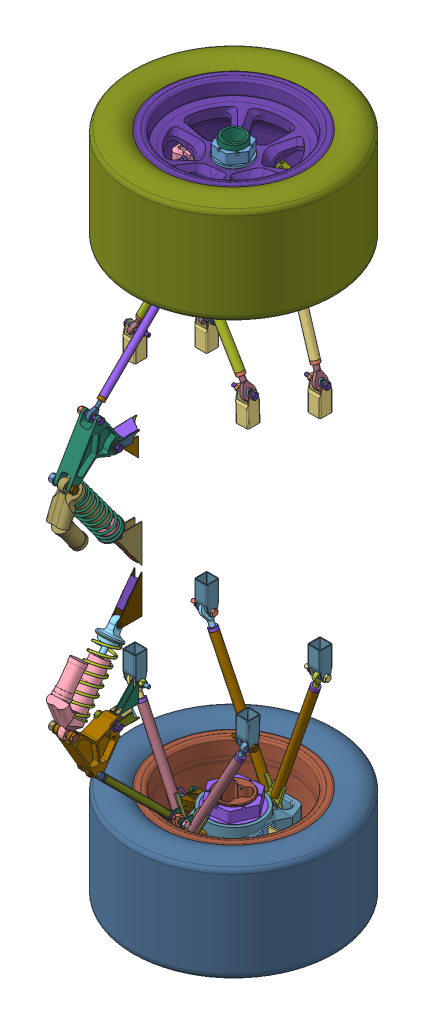
SolidWorks assembly UN-A1001-AB-Rear Unsprung Assembly, configuration Default. Lengths in mm.
Overall size (411.48 1363.58 600.2).
282 component instances, 147 part files, 8 mates.
Components (placement in the parent):
- SP-A0200-AH-Rear Axle Assembly-1: SP-A0200-AH-Rear Axle Assembly [Default] at origin size (274.88 563.57 484.64)
  - SP-AA-Rear Lower A-Arm^SP-A0200-AH-Rear Axle Assembly-1: SP-AA-Rear Lower A-Arm^SP-A0200-AH-Rear Axle Assembly [Default] at (0 -0.399 0.6588) x (1 0 0) z (0 0.002866 0.999996) size (222.76 290.57 36.42) (virtual)
    - SP-Lower Apex Rear-1: SP-Lower Apex Rear [Default] at (-792.4265 549.6462 121.5417) x (-0.932505 -0.360479 0.022123) z (0 -0.061256 -0.998122) size (54.94 63.8 9.53)
    - MirrorFS-MALE ROD END UNF-3A, 0.3125x24-0.25D (XAM-4)1-1: MirrorFS-MALE ROD END UNF-3A, 0.3125x24-0.25D (XAM-4)1 [Default] at (-906.7265 255.0788 139.6197) x (0.932505 -0.360479 0.022123) z (-0.361157 -0.930754 0.057121)
    - MirrorFS-MALE ROD END UNF-3A, 0.3125x24-0.25D (XAM-4)1-2: MirrorFS-MALE ROD END UNF-3A, 0.3125x24-0.25D (XAM-4)1 [Default] at (-678.1265 255.0788 139.6197) x (0.932505 0.360479 -0.022123) z (0.361157 -0.930754 0.057121)
    - SP-10003-AB-Threaded Insert-1: SP-10003-AB-Threaded Insert [A-Arm] at (-890.6731 296.4508 137.0806) x (0.932505 -0.360479 0.022123) z (-0.361157 -0.930754 0.057121) size (15.88 15.88 15.88)
    - SP-10003-AB-Threaded Insert-2: SP-10003-AB-Threaded Insert [A-Arm] at (-694.18 296.4508 137.0806) x (0.932505 0.360479 -0.022123) z (0.361157 -0.930754 0.057121) size (15.88 15.88 15.88)
    - SP-Rear Lower A-Arm Tube-1: SP-Rear Lower A-Arm Tube [Default] at (-838.6322 430.5677 128.8497) x (-0.361157 -0.930754 0.057121) z (0 -0.061256 -0.998122) size (257.84 15.88 15.88)
    - SP-Rear Lower A-Arm Tube-2: SP-Rear Lower A-Arm Tube [Default] at (-746.2209 430.5677 128.8497) x (0.361157 -0.930754 0.057121) z (0 0.061256 0.998122) size (257.84 15.88 15.88)
    - FS-HIGH MISALIGN SPHERICAL BEARING, 0.375-0.906D (3072-6G)-1: FS-HIGH MISALIGN SPHERICAL BEARING, 0.375-0.906D (3072-6G) [Default] at (-792.4265 549.6462 121.5417) x (-0.932505 0.360479 -0.022123) z (-0.361157 -0.930754 0.057121) size (26.46 21.71 26.13)
      - Race^FS-HIGH MISALIGN SPHERICAL BEARING, 0.375-0.906D (3072-6G)-1: Race^FS-HIGH MISALIGN SPHERICAL BEARING, 0.375-0.906D (3072-6G) [Default] at origin size (23.01 8.76 23.01) (virtual)
      - Ball^FS-HIGH MISALIGN SPHERICAL BEARING, 0.375-0.906D (3072-6G)-1: Ball^FS-HIGH MISALIGN SPHERICAL BEARING, 0.375-0.906D (3072-6G) [Default] x (0.359576 -0.008176 0.93308) z (-0.932238 -0.046516 0.358844) size (19.84 20.65 19.84) (virtual)
  - SP-AA-Rear Upper A-Arm^SP-A0200-AH-Rear Axle Assembly-1: SP-AA-Rear Upper A-Arm^SP-A0200-AH-Rear Axle Assembly [Default] at (-38.1 -1.9308 1.9372) x (1 0 0) z (0 0.00685 0.999977) size (216 215.55 29.43) (virtual)
    - SP-Upper Apex Rear-1: SP-Upper Apex Rear [Default] at (-755.8405 523.8827 293.8505) x (0.884705 -0.465567 -0.023329) z (0 -0.050046 0.998747) size (76.45 83.12 9.53)
    - MirrorFS-MALE ROD END UNF-3A, 0.3125x24-0.25D (XAM-4)1-1: MirrorFS-MALE ROD END UNF-3A, 0.3125x24-0.25D (XAM-4)1 [Default] at (-870.1405 307.2255 282.9942) x (0.884705 -0.465567 -0.023329) z (-0.466151 -0.883596 -0.044276)
    - MirrorFS-MALE ROD END UNF-3A, 0.3125x24-0.25D (XAM-4)1-2: MirrorFS-MALE ROD END UNF-3A, 0.3125x24-0.25D (XAM-4)1 [Default] at (-641.5405 307.2255 282.9942) x (0.884705 0.465567 0.023329) z (0.466151 -0.883596 -0.044276)
    - SP-10003-AB-Threaded Insert-1: SP-10003-AB-Threaded Insert [A-Arm] at (-849.4201 346.5014 284.9623) x (0.884705 -0.465567 -0.023329) z (-0.466151 -0.883596 -0.044276) size (15.88 15.88 15.88)
    - SP-10003-AB-Threaded Insert-2: SP-10003-AB-Threaded Insert [A-Arm] at (-662.261 346.5014 284.9623) x (0.884705 0.465567 0.023329) z (0.466151 -0.883596 -0.044276) size (15.88 15.88 15.88)
    - SP-Rear Upper A-Arm Tube-1: SP-Rear Upper A-Arm Tube [Default] at (-812.9905 415.5541 288.4224) x (0.466151 0.883596 0.044276) z (0.884705 -0.465567 -0.023329) size (186.28 15.88 15.88)
    - SP-Rear Upper A-Arm Tube-2: SP-Rear Upper A-Arm Tube [Default] at (-698.6905 415.5541 288.4224) x (-0.466151 0.883596 0.044276) z (0.884705 0.465567 0.023329) size (186.28 15.88 15.88)
    - FS-HIGH MISALIGN SPHERICAL BEARING, 0.375-0.906D (3072-6G)-1: FS-HIGH MISALIGN SPHERICAL BEARING, 0.375-0.906D (3072-6G) [Default] at (-755.8405 523.8827 293.8505) x (0.884705 -0.465567 -0.023329) z (-0.466151 -0.883596 -0.044276) size (26.46 21.71 26.13)
      - Race^FS-HIGH MISALIGN SPHERICAL BEARING, 0.375-0.906D (3072-6G)-1: Race^FS-HIGH MISALIGN SPHERICAL BEARING, 0.375-0.906D (3072-6G) [Default] at origin size (23.01 8.76 23.01) (virtual)
      - Ball^FS-HIGH MISALIGN SPHERICAL BEARING, 0.375-0.906D (3072-6G)-1: Ball^FS-HIGH MISALIGN SPHERICAL BEARING, 0.375-0.906D (3072-6G) [Default] x (0.359576 -0.008176 0.93308) z (-0.932238 -0.046516 0.358844) size (19.84 20.65 19.84) (virtual)
  - Assem8^SP-A0200-AH-Rear Axle Assembly-1: Assem8^SP-A0200-AH-Rear Axle Assembly [Default] at (-1592.9214 814.7933 712.2762) x (-0.999891 -0.01037 0.010464) z (0.012143 -0.982316 0.186836) size (17.98 166.51 230.13) (virtual)
    - Part2^Assem8_SP-A0200-AH-Rear Axle Assembly-1: Part2^Assem8_SP-A0200-AH-Rear Axle Assembly [Default] at origin size (15.39 113.92 157.78) (virtual)
    - SP-10003-AC-Threaded Insert-2: SP-10003-AC-Threaded Insert [AM-4 Rod End Thread] at (-799.064 427.6015 294.0449) x (-0.999891 -0.008342 0.012143) z (-0.014733 0.566176 -0.824153) size (12.7 12.7 15.88)
    - SP-10003-AC-Threaded Insert-3: SP-10003-AC-Threaded Insert [AM-4 Rod End Thread] at (-796.6527 334.9355 428.9338) x (-0.999891 -0.008342 0.012143) z (0.014733 -0.566176 0.824153) size (12.7 12.7 15.88)
    - FS-MALE ROD END UNF-3A, 0.25x28-0.25D (AM-4)-1: FS-MALE ROD END UNF-3A, 0.25x28-0.25D (AM-4) [Default] at (-796.0446 311.5665 462.9507) x (0 -0.824242 -0.566238) z (-0.014733 0.566176 -0.824153) size (19.32 14.06 49.44)
      - Body^FS-MALE ROD END UNF-3A, 0.25x28-0.25D (AM-4)-2: Body^FS-MALE ROD END UNF-3A, 0.25x28-0.25D (AM-4) [Default] at origin size (19.32 7.2 49.44) (virtual)
      - Ball^FS-MALE ROD END UNF-3A, 0.25x28-0.25D (AM-4)-2: Ball^FS-MALE ROD END UNF-3A, 0.25x28-0.25D (AM-4) [Default] x (0.09633 0.218783 0.971007) z (-0.984027 0.167661 0.059845) size (12.7 9.53 12.7) (virtual)
    - FS-MALE ROD END UNF-3A, 0.25x28-0.25D (AM-4)-2: FS-MALE ROD END UNF-3A, 0.25x28-0.25D (AM-4) [Default] at (-799.6721 450.9704 260.028) x (0 -0.824242 -0.566238) z (0.014733 -0.566176 0.824153) size (19.32 14.06 49.44)
      - Body^FS-MALE ROD END UNF-3A, 0.25x28-0.25D (AM-4)-2: Body^FS-MALE ROD END UNF-3A, 0.25x28-0.25D (AM-4) [Default] at origin size (19.32 7.2 49.44) (virtual)
      - Ball^FS-MALE ROD END UNF-3A, 0.25x28-0.25D (AM-4)-2: Ball^FS-MALE ROD END UNF-3A, 0.25x28-0.25D (AM-4) [Default] x (0.09633 0.218783 0.971007) z (-0.984027 0.167661 0.059845) size (12.7 9.53 12.7) (virtual)
  - SP-A0105-AC-Ohlin TTX25 MKII, 200mm-1: SP-A0105-AC-Ohlin TTX25 MKII, 200mm [Default] at (-793.9406 216.4917 537.8809) x (-1 0 0) z (0 0.803503 0.5953) size (48.39 85.02 197.6)
    - Shock Body^SP-A0105-AC-Ohlin TTX25 MKII, 200mm-1: Shock Body^SP-A0105-AC-Ohlin TTX25 MKII, 200mm [Default] at origin size (40.76 80 131.7) (virtual)
    - Head^SP-A0105-AC-Ohlin TTX25 MKII, 200mm-1: Head^SP-A0105-AC-Ohlin TTX25 MKII, 200mm [Default] at (0 0 -174.6) size (46 46 119) (virtual)
    - Ball^SP-A0105-AC-Ohlin TTX25 MKII, 200mm-1: Ball^SP-A0105-AC-Ohlin TTX25 MKII, 200mm [Default] at (0 0 -174.6) x (-0.011681 0.107343 0.994153) z (0.993776 0.111394 -0.000351) size (15 15 8) (virtual)
    - Ball^SP-A0105-AC-Ohlin TTX25 MKII, 200mm-2: Ball^SP-A0105-AC-Ohlin TTX25 MKII, 200mm [Default] x (0.079523 -0.862756 -0.499328) z (0.965926 -0.057074 0.252448) size (15 15 8) (virtual)
    - SP-#####-AB-Spring-1: SP-#####-AB-Spring [Default] at (0 0 -151.1) size (48.39 49.05 127.97)
  - FS-BALL BEARING, 0.25ID-0.75OD (60355K702)-1: FS-BALL BEARING, 0.25ID-0.75OD (60355K702) [Default] at (-784.8125 243.84 446.6415) x (0 -0.287121 0.957894) z (-1 0 0) size (19.05 19.05 7.14)
  - FS-BALL BEARING, 0.25ID-0.75OD (60355K702)-2: FS-BALL BEARING, 0.25ID-0.75OD (60355K702) [Default] at (-803.0688 243.84 446.6415) x (0 0.287121 -0.957894) z (1 0 0) size (19.05 19.05 7.14)
  - FS-CADMIUM PLATED C3 HEX, 0.25x28-1.65-0.469 (AN4-13A)-2: FS-CADMIUM PLATED C3 HEX, 0.25x28-1.65-0.469 (AN4-13A) [Default] at (-796.8362 310.0391 484.3789) x (-1 0 0) z (0 0.868755 0.495242) size (46.28 12.9 11.18)
  - FS-ZINC YELLOW CHROMATE C10.9 HX, M8x1.25-40-22 (95327A569)-1: FS-ZINC YELLOW CHROMATE C10.9 HX, M8x1.25-40-22 (95327A569) [Default] at (-795.4156 216.4917 537.8809) x (-1 0 0) z (0 -0.287121 0.957894) size (45.3 15.01 13)
  - FS-NYLOC FLHX C8, M8x1.25-11.1 (92461A400)-1: FS-NYLOC FLHX C8, M8x1.25-11.1 (92461A400) [Default] at (-820.9156 216.4917 537.8809) x (0 0.868058 -0.496463) z (-1 0 0) size (17.9 17.9 11.1)
  - FS-NYLOC G8 HX, 0.25x28-0.3125 (90630A145)-1: FS-NYLOC G8 HX, 0.25x28-0.3125 (90630A145) [Default] at (-809.8156 310.0391 484.3789) x (0 0.868058 -0.496463) z (0 0.496463 0.868058) size (11.11 7.94 12.83)
  - SP-C30066-AA-A-Arm Tab Box-1: SP-C30066-AA-A-Arm Tab Box [Default] at (-680.9758 289.7175 282.8202) x (-0.029021 0.999579 0) z (0 0 -1) size (60.32 25.4 25.4)
  - SP-C30066-AA-A-Arm Tab Box-2: SP-C30066-AA-A-Arm Tab Box [Default] at (-908.2405 289.7636 282.8202) x (0 1 0) z (0 0 -1) size (60.32 25.4 25.4)
  - SP-C30066-AA-A-Arm Tab Box-3: SP-C30066-AA-A-Arm Tab Box [Default] at (-678.1265 237.6164 139.5469) x (0 1 0) z (0 0 1) size (60.32 25.4 25.4)
  - SP-C30066-AA-A-Arm Tab Box-4: SP-C30066-AA-A-Arm Tab Box [Default] at (-906.7265 237.6164 139.5469) x (0 1 0) z (0 0 1) size (60.32 25.4 25.4)
  - MirrorSP-30063-AB-Pushrod Tab-1: MirrorSP-30063-AB-Pushrod Tab [Default] at (-782.0343 483.2134 293.6084) x (1 0 0) z (0 0.043203 -0.999066) size (1.59 15.88 23.81)
  - MirrorSP-30063-AB-Pushrod Tab-2: MirrorSP-30063-AB-Pushrod Tab [Default] at (-805.8468 483.2134 293.6084) x (-1 0 0) z (0 0.043203 -0.999066) size (1.59 15.88 23.81)
  - FS-NYLOC FLHX C8, M8x1.25-11.1 (92461A400)-2: FS-NYLOC FLHX C8, M8x1.25-11.1 (92461A400) [Default] at (-820.9156 243.84 446.6415) x (0 0 -1) z (-1 0 0) size (17.9 17.9 11.1)
  - FS-CADMIUM PLATED C3 HEX, 0.25x28-1.65-0.469 (AN4-13A)-3: FS-CADMIUM PLATED C3 HEX, 0.25x28-1.65-0.469 (AN4-13A) [Default] at (-796.8362 243.84 446.6415) x (-1 0 0) z (0 0.287121 -0.957894) size (46.28 12.9 11.18)
  - FS-CADMIUM PLATED C3 HEX, 0.25x28-1.65-0.469 (AN4-13A)-4: FS-CADMIUM PLATED C3 HEX, 0.25x28-1.65-0.469 (AN4-13A) [Default] at (-687.5506 306.9965 282.8202) x (-0.999579 -0.029021 0) z (0 0 -1) size (46.28 12.9 11.18)
  - FS-CADMIUM PLATED C3 HEX, 0.25x28-1.65-0.469 (AN4-13A)-5: FS-CADMIUM PLATED C3 HEX, 0.25x28-1.65-0.469 (AN4-13A) [Default] at (-902.1699 307.2261 282.8202) size (46.28 12.9 11.18)
  - FS-CADMIUM PLATED C3 HEX, 0.25x28-1.65-0.469 (AN4-13A)-6: FS-CADMIUM PLATED C3 HEX, 0.25x28-1.65-0.469 (AN4-13A) [Default] at (-912.7971 255.0789 139.5469) x (-1 0 0) z (0 0 -1) size (46.28 12.9 11.18)
  - FS-CADMIUM PLATED C3 HEX, 0.25x28-1.65-0.469 (AN4-13A)-7: FS-CADMIUM PLATED C3 HEX, 0.25x28-1.65-0.469 (AN4-13A) [Default] at (-684.1971 255.0789 139.5469) x (-1 0 0) z (0 0 -1) size (46.28 12.9 11.18)
  - FS-CADMIUM PLATED C3 HEX, 0.25x28-1.65-0.469 (AN4-13A)-8: FS-CADMIUM PLATED C3 HEX, 0.25x28-1.65-0.469 (AN4-13A) [Default] at (-799.2174 482.5275 309.4686) x (-1 0 0) z (0 -0.609051 0.793131) size (46.28 12.9 11.18)
  - FS-NYLOC G8 HX, 0.25x28-0.3125 (90630A145)-3: FS-NYLOC G8 HX, 0.25x28-0.3125 (90630A145) [Default] at (-807.4343 482.5275 309.4686) x (0 -0.043203 0.999066) z (0 -0.999066 -0.043203) size (11.11 7.94 12.83)
  - FS-NYLOC G8 HX, 0.25x28-0.3125 (90630A145)-4: FS-NYLOC G8 HX, 0.25x28-0.3125 (90630A145) [Default] at (-694.1772 306.8041 282.8202) x (-0.029021 0.999579 0) z (0 0 1) size (11.11 7.94 12.83)
  - FS-NYLOC G8 HX, 0.25x28-0.3125 (90630A145)-5: FS-NYLOC G8 HX, 0.25x28-0.3125 (90630A145) [Default] at (-895.5405 307.2261 282.8202) x (0 1 0) z (0 0 -1) size (11.11 7.94 12.83)
  - FS-NYLOC G8 HX, 0.25x28-0.3125 (90630A145)-6: FS-NYLOC G8 HX, 0.25x28-0.3125 (90630A145) [Default] at (-919.4265 255.0789 139.5469) x (0 1 0) z (0 0 1) size (11.11 7.94 12.83)
  - FS-NYLOC G8 HX, 0.25x28-0.3125 (90630A145)-7: FS-NYLOC G8 HX, 0.25x28-0.3125 (90630A145) [Default] at (-690.8265 255.0789 139.5469) x (0 -1 0) z (0 0 -1) size (11.11 7.94 12.83)
  - FS-ROD END RETAINING WASHER, 0.25-0.245 (NO PN)-5: FS-ROD END RETAINING WASHER, 0.25-0.245 (NO PN) [Default] at (-781.9073 482.5275 309.4686) x (0 1 0) z (-1 0 0) size (12.7 12.7 6.22)
  - FS-ROD END RETAINING WASHER, 0.25-0.245 (NO PN)-6: FS-ROD END RETAINING WASHER, 0.25-0.245 (NO PN) [Default] at (-805.9738 482.5275 309.4686) x (0 0.978954 0.204082) z (1 0 0) size (12.7 12.7 6.22)
  - SP-A0200-Rear Inner Rocker Gusset-1: SP-A0200-Rear Inner Rocker Gusset [Default] at (-793.9406 234.6955 425.4808) x (1 0 0) z (0 0.052336 0.99863) size (26.99 1.59 48.67)
  - SP-A0200-Rear Long Rocker Tab-1: SP-A0200-Rear Long Rocker Tab [Rear] at (-807.4344 243.84 446.6415) x (1 0 0) z (0 -0.00621 -0.999981) size (1.59 19.05 73.11)
  - SP-A0200-Rear Outer Rocker Gusset-1: SP-A0200-Rear Outer Rocker Gusset [Default] at (-793.9406 251.3902 418.9606) x (1 0 0) z (0 -0.039929 0.999203) size (26.99 1.59 43.52)
  - SP-A0200-Rear Rocker Gusset Support-1: SP-A0200-Rear Rocker Gusset Support [Default] at (-800.2906 228.5949 403.7833) x (0 0 1) z (0 1 0) size (38.05 1.59 40.09)
  - SP-A0200-Rear Short Rocker Tab-1: SP-A0200-Rear Short Rocker Tab [Rear] at (-780.4469 243.8408 446.6212) x (1 0 0) z (0 -0.00621 -0.999981) size (1.59 17.17 50.59)
  - SP-A0200-Rear Rocker Gusset Support-2: SP-A0200-Rear Rocker Gusset Support [Default] at (-789.8131 228.5949 403.7833) x (0 0 1) z (0 1 0) size (38.05 1.59 40.09)
  - SP-A0200-Rear Shock Gusset-1: SP-A0200-Rear Shock Gusset [Default] at (-793.9406 34.3591 413.4634) x (1 0 0) z (0 0.809017 0.587785) size (14.29 1.59 50.8)
  - SP-A0200-Rear Shock Tab-1: SP-A0200-Rear Shock Tab [Rear] at (-786.7969 76.2 433.9415) x (-1 0 0) z (0 -0.809017 -0.587785) size (1.59 45.95 88.76)
  - SP-A0200-Rear Shock Tab-2: SP-A0200-Rear Shock Tab [Front] at (-801.0844 76.2 433.9415) x (-1 0 0) z (0 -0.809017 -0.587785) size (1.59 45.95 88.76)
  - FS-MALE ROD END UNJF-3A, 0.375x24-0.25D (HXAM-4T)-4: FS-MALE ROD END UNJF-3A, 0.375x24-0.25D (HXAM-4T) [Simplified] at (-679.6405 307.2261 282.8202) x (0 0.043203 -0.999066) z (-0.466151 0.883879 0.038222) size (26.22 15.06 62.54)
    - Body^FS-MALE ROD END UNJF-3A, 0.375x24-0.25D (HXAM-4T)-1: Body^FS-MALE ROD END UNJF-3A, 0.375x24-0.25D (HXAM-4T) [no_threads] at origin size (26.22 9.62 62.54)
    - Ball^FS-MALE ROD END UNJF-3A, 0.375x24-0.25D (HXAM-4T)-1: Ball^FS-MALE ROD END UNJF-3A, 0.375x24-0.25D (HXAM-4T) [Default] at origin size (15.06 15.06 15.06)
  - FS-MALE ROD END UNJF-3A, 0.375x24-0.25D (HXAM-4T)-5: FS-MALE ROD END UNJF-3A, 0.375x24-0.25D (HXAM-4T) [Simplified] at (-908.2405 307.2261 282.8202) x (0 -0.043203 0.999066) z (0.466151 0.883879 0.038222) size (26.22 15.06 62.54)
    - Body^FS-MALE ROD END UNJF-3A, 0.375x24-0.25D (HXAM-4T)-1: Body^FS-MALE ROD END UNJF-3A, 0.375x24-0.25D (HXAM-4T) [no_threads] at origin size (26.22 9.62 62.54)
    - Ball^FS-MALE ROD END UNJF-3A, 0.375x24-0.25D (HXAM-4T)-1: Ball^FS-MALE ROD END UNJF-3A, 0.375x24-0.25D (HXAM-4T) [Default] at origin size (15.06 15.06 15.06)
  - FS-MALE ROD END UNJF-3A, 0.375x24-0.25D (HXAM-4T)-6: FS-MALE ROD END UNJF-3A, 0.375x24-0.25D (HXAM-4T) [Simplified] at (-906.7265 255.0789 139.5469) x (0 0.064116 0.997942) z (0.361157 0.930586 -0.059789) size (26.22 15.06 62.54)
    - Body^FS-MALE ROD END UNJF-3A, 0.375x24-0.25D (HXAM-4T)-1: Body^FS-MALE ROD END UNJF-3A, 0.375x24-0.25D (HXAM-4T) [no_threads] at origin size (26.22 9.62 62.54)
    - Ball^FS-MALE ROD END UNJF-3A, 0.375x24-0.25D (HXAM-4T)-1: Ball^FS-MALE ROD END UNJF-3A, 0.375x24-0.25D (HXAM-4T) [Default] at origin size (15.06 15.06 15.06)
  - FS-MALE ROD END UNJF-3A, 0.375x24-0.25D (HXAM-4T)-7: FS-MALE ROD END UNJF-3A, 0.375x24-0.25D (HXAM-4T) [Simplified] at (-678.1265 255.0789 139.5469) x (0 -0.064116 -0.997942) z (-0.361157 0.930586 -0.059789) size (26.22 15.06 62.54)
    - Body^FS-MALE ROD END UNJF-3A, 0.375x24-0.25D (HXAM-4T)-1: Body^FS-MALE ROD END UNJF-3A, 0.375x24-0.25D (HXAM-4T) [no_threads] at origin size (26.22 9.62 62.54)
    - Ball^FS-MALE ROD END UNJF-3A, 0.375x24-0.25D (HXAM-4T)-1: Ball^FS-MALE ROD END UNJF-3A, 0.375x24-0.25D (HXAM-4T) [Default] at origin size (15.06 15.06 15.06)
  - SP-B0100-Rear Rocker-1: SP-B0100-Rear Rocker [Default] at (14.7593 458.8134 -310.4211) x (0.993764 -0.111506 -0.000215) z (-0.085107 -0.759728 0.644647) size (43.51 92.41 122.03)
- WT-A0100-XG-Corner Assembly-1: WT-A0100-XG-Corner Assembly [Front Left Corner Assembly] at origin size (260.47 172.81 260.47)
  - WT-00202-AA-Hoosier R25B 16x7_5-10-1: WT-00202-AA-Hoosier R25B 16x7_5-10 [Default] at (-793.1174 574.9879 198.909) x (-1 0 0) z (0 -1 0.000253) size (411.48 411.48 213.5)
  - WT-00201-AA-OZ Centerlock 10in Wheel-1: WT-00201-AA-OZ Centerlock 10in Wheel [Default] at (-793.1174 596.9879 198.9034) x (-0.992442 0.000031 0.122714) z (0 1 -0.000253) size (288.79 288.79 189.86)
  - WT-10105-AA-Drive Pin-8: WT-10105-AA-Drive Pin [Default] at (-825.0424 596.994 223.0032) x (-0.121576 0.000251 0.992582) z (-0.992582 -0.000031 -0.121576) size (12.67 23.01 11.95)
  - WT-10102-AA-Centerlock Nut-1: WT-10102-AA-Centerlock Nut [Default] at (-793.1174 647.6073 198.8906) x (-0.440541 -0.000227 -0.897732) z (0.897733 -0.000111 -0.440541) size (66 31.75 66)
  - WT-XF-Upright-1: WT-XF-Upright [Default] at (-793.1174 537.8923 198.9183) x (-0.999961 -0.000002 -0.008824) z (-0.008824 0.000253 0.999961) size (134.42 50.23 211.08)
  - BR-A0102-AA-Caliper Assembly-1: BR-A0102-AA-Caliper Assembly [Default] at (-874.0145 570.8565 194.5235) x (-0.069854 0.000252 0.997557) z (0 -1 0.000253) size (40.11 43.54 52.73)
    - cp3838-M08x1.25m_CP4477-110^BR-A0102-AA-Caliper Assembly-1: cp3838-M08x1.25m_CP4477-110^BR-A0102-AA-Caliper Assembly [Default] at (-13.37 19.3 19.55) x (-0.999952 -0.009843 0) z (0 0 -1) size (13 13 46) (virtual)
    - CP4226-102^BR-A0102-AA-Caliper Assembly-1: CP4226-102^BR-A0102-AA-Caliper Assembly [Default] x (-1 0 0) z (0 0 -1) size (63.87 47.42 31.57) (virtual)
    - cp4226-104_CP4226-104^BR-A0102-AA-Caliper Assembly-1: cp4226-104_CP4226-104^BR-A0102-AA-Caliper Assembly [Default] at (0 23 -31.9644) x (0 0 1) z (-1 0 0) size (61.35 20.1 3) (virtual)
    - CP4226-101^BR-A0102-AA-Caliper Assembly-1: CP4226-101^BR-A0102-AA-Caliper Assembly [Default] at origin size (81.26 55.69 34.68) (virtual)
    - cp3838-M08x1.25m_CP4477-110^BR-A0102-AA-Caliper Assembly-2: cp3838-M08x1.25m_CP4477-110^BR-A0102-AA-Caliper Assembly [Default] at (13.37 19.3 19.55) x (-0.997666 -0.068288 0) z (0 0 -1) size (13 13 46) (virtual)
    - cp3049-40a_CP4226-103^BR-A0102-AA-Caliper Assembly-1: cp3049-40a_CP4226-103^BR-A0102-AA-Caliper Assembly [Default] at (0 0 10.305) x (-0.993137 0.116957 0) z (0 0 -1) size (25.2 25.2 14.87) (virtual)
    - CP4469-101^BR-A0102-AA-Caliper Assembly-1: CP4469-101^BR-A0102-AA-Caliper Assembly [Default] at (42 -11.5 -23.98) x (0 -0.520643 0.853775) z (-1 0 0) size (9.18 8.2 29.15) (virtual)
    - cp3049-40a_CP4226-103^BR-A0102-AA-Caliper Assembly-2: cp3049-40a_CP4226-103^BR-A0102-AA-Caliper Assembly [Default] at (0 0 -10.305) size (25.2 25.2 14.87) (virtual)
    - Brake Pad^BR-A0102-AA-Caliper Assembly-1: Brake Pad^BR-A0102-AA-Caliper Assembly [Default] at (0 11.1798 8.5855) x (-1 0 0) z (0 -1 0) size (39.62 6.86 43.54) (virtual)
    - Brake Pad^BR-A0102-AA-Caliper Assembly-2: Brake Pad^BR-A0102-AA-Caliper Assembly [Default] at (0 11.1798 -8.5905) x (1 0 0) z (0 -1 0) size (39.62 6.86 43.54) (virtual)
  - WT-10103-AA-Grease Seal-1: WT-10103-AA-Grease Seal [Default] at (-793.1174 559.091 198.913) x (-0.781145 -0.000158 -0.624349) z (-0.624349 0.000198 0.781145) size (97.66 13.92 97.66)
  - LL713049-LL713010-TheTimkenCompany-3D-11-03-2022.stp-1: LL713049-LL713010-TheTimkenCompany-3D-11-03-2022.stp [Default] at (-793.1174 541.0673 198.9175) x (0 1 -0.000253) z (0.586717 -0.000205 -0.809792) size (15.53 98.42 98.42)
  - LL713049-LL713010-TheTimkenCompany-3D-11-03-2022.stp-2: LL713049-LL713010-TheTimkenCompany-3D-11-03-2022.stp [Default] at (-793.1174 534.7173 198.9191) x (0 -1 0.000253) z (0.531557 -0.000214 -0.847022) size (15.53 98.42 98.42)
  - WT-XA-Tripod Nut-1: WT-XA-Tripod Nut [Default] at (-793.1174 516.4598 198.9238) x (0 1 -0.000253) z (0.798123 -0.000152 -0.602494) size (30.44 98.37 98.37)
  - WT-BA-Camber Block-1: WT-BA-Camber Block [Default] at (-793.95 547.3609 293.2547) x (-0.999961 -0.000002 -0.008824) z (-0.008819 -0.034647 0.999361) size (82.61 35.93 35.38)
  - 91290A442_Alloy Steel Socket Head Screw-1: 91290A442_Alloy Steel Socket Head Screw [91290A442] at (-816.177 556.8302 293.3869) x (0.914102 0.014329 -0.405231) z (0.000308 -0.9994 -0.034645) size (13 13 48.09)
  - BR-A0000-AB-Rear Brake Assembly-1: BR-A0000-AB-Rear Brake Assembly [Default No Bobbins] at (-793.1174 596.9879 198.9034) x (-0.602494 -0.000202 -0.798123) z (-0.798123 0.000152 0.602494) size (251.55 172.72 251.55)
    - WT-XA-#####-Tripod Hub-2: WT-XA-#####-Tripod Hub [Default] at origin size (102.86 172.72 102.86)
    - BR-20601-AB-Brake Rotor-1: BR-20601-AB-Brake Rotor [Default] at (0 26.1303 0) x (0.866025 0 -0.5) z (0.5 0 0.866025) size (184.15 4.76 184.15)
    - BR-20603-BA-Floating Bobbins-1: BR-20603-BA-Floating Bobbins [Default] at (39.8696 25.9874 23.0188) size (15.88 8.92 15.88)
    - BR-20603-BA-Floating Bobbins-2: BR-20603-BA-Floating Bobbins [Default] at (0 25.9874 46.0375) x (0.5 0 0.866025) z (-0.866025 0 0.5) size (15.88 8.92 15.88)
    - BR-20603-BA-Floating Bobbins-3: BR-20603-BA-Floating Bobbins [Default] at (-39.8696 25.9874 23.0188) x (-0.5 0 0.866025) z (-0.866025 0 -0.5) size (15.88 8.92 15.88)
    - BR-20603-BA-Floating Bobbins-4: BR-20603-BA-Floating Bobbins [Default] at (-39.8696 25.9874 -23.0188) x (-1 0 0) z (0 0 -1) size (15.88 8.92 15.88)
    - BR-20603-BA-Floating Bobbins-5: BR-20603-BA-Floating Bobbins [Default] at (0 25.9874 -46.0375) x (-0.5 0 -0.866025) z (0.866025 0 -0.5) size (15.88 8.92 15.88)
    - BR-20603-BA-Floating Bobbins-6: BR-20603-BA-Floating Bobbins [Default] at (39.8696 25.9874 -23.0188) x (0.5 0 -0.866025) z (0.866025 0 0.5) size (15.88 8.92 15.88)
    - WT-20104-AB-Rear Sensor Ring-1: WT-20104-AB-Rear Sensor Ring [Default] at (0 30.099 0) x (0.882948 0 -0.469472) z (0 -1 0) size (137 137 1.59)
    - 91590A121_External Retaining Ring-1: 91590A121_External Retaining Ring [91590A121] at (-39.8696 29.2354 23.0188) x (0 1 0) z (-0.857167 0 0.515038) size (0.64 14.63 13.25)
    - 91590A121_External Retaining Ring-2: 91590A121_External Retaining Ring [91590A121] at (-39.8696 29.2354 -23.0188) x (0 1 0) z (-0.87462 0 -0.48481) size (0.64 14.63 13.25)
    - 91590A121_External Retaining Ring-3: 91590A121_External Retaining Ring [91590A121] at (0 29.2354 -46.0375) x (0 1 0) z (-0.017452 0 -0.999848) size (0.64 14.63 13.25)
    - 91590A121_External Retaining Ring-4: 91590A121_External Retaining Ring [91590A121] at (39.8696 29.2354 -23.0188) x (0 1 0) z (0.857167 0 -0.515038) size (0.64 14.63 13.25)
    - 91590A121_External Retaining Ring-5: 91590A121_External Retaining Ring [91590A121] at (39.8696 29.2354 23.0188) x (0 1 0) z (0.87462 0 0.48481) size (0.64 14.63 13.25)
    - 91590A121_External Retaining Ring-6: 91590A121_External Retaining Ring [91590A121] at (0 29.2354 46.0375) x (0 1 0) z (0.017452 0 0.999848) size (0.64 14.63 13.25)
    - 97447A110_Aluminum Blind Rivets with Aluminum Mandrel-1: 97447A110_Aluminum Blind Rivets with Aluminum Mandrel [97447A110] at (9.6137 30.099 51.8707) x (-0.302097 0 -0.953277) z (0 1 0) size (5.03 5.03 11.56)
    - 97447A110_Aluminum Blind Rivets with Aluminum Mandrel-2: 97447A110_Aluminum Blind Rivets with Aluminum Mandrel [97447A110] at (-40.1145 30.099 34.261) x (0.674514 0 -0.738262) z (0 1 0) size (5.03 5.03 11.56)
    - 97447A110_Aluminum Blind Rivets with Aluminum Mandrel-3: 97447A110_Aluminum Blind Rivets with Aluminum Mandrel [97447A110] at (-49.7282 30.099 -17.6097) x (0.976611 0 0.215015) z (0 1 0) size (5.03 5.03 11.56)
    - 97447A110_Aluminum Blind Rivets with Aluminum Mandrel-4: 97447A110_Aluminum Blind Rivets with Aluminum Mandrel [97447A110] at (-9.6137 30.099 -51.8707) x (0.302097 0 0.953277) z (0 1 0) size (5.03 5.03 11.56)
    - 97447A110_Aluminum Blind Rivets with Aluminum Mandrel-5: 97447A110_Aluminum Blind Rivets with Aluminum Mandrel [97447A110] at (40.1145 30.099 -34.261) x (-0.674514 0 0.738262) z (0 1 0) size (5.03 5.03 11.56)
    - 97447A110_Aluminum Blind Rivets with Aluminum Mandrel-6: 97447A110_Aluminum Blind Rivets with Aluminum Mandrel [97447A110] at (49.7282 30.099 17.6097) x (-0.976611 0 -0.215015) z (0 1 0) size (5.03 5.03 11.56)
  - FS-Jet Nut, M8x1.25 (MJET-M8X1.25)-1: FS-Jet Nut, M8x1.25 (MJET-M8X1.25) [Default] at (-816.1783 561.0546 293.5333) x (-0.906747 0.01433 -0.421432) z (-0.000308 0.9994 0.034645) size (13.6 13.6 7)
  - 91290A442_Alloy Steel Socket Head Screw-2: 91290A442_Alloy Steel Socket Head Screw [91290A442] at (-771.7287 556.8303 293.7791) x (-0.549228 0.028783 -0.835176) z (0.000308 -0.9994 -0.034645) size (13 13 48.09)
  - FS-Jet Nut, M8x1.25 (MJET-M8X1.25)-2: FS-Jet Nut, M8x1.25 (MJET-M8X1.25) [Default] at (-771.73 561.0547 293.9256) x (0.139109 0.034351 -0.989681) z (-0.000308 0.9994 0.034645) size (13.6 13.6 7)
  - WT-10105-AA-Drive Pin-21: WT-10105-AA-Drive Pin [Default] at (-769.0177 596.9959 230.8283) x (0.992582 0.000031 0.121576) z (-0.121576 0.000251 0.992582) size (12.67 23.01 11.95)
  - WT-10105-AA-Drive Pin-22: WT-10105-AA-Drive Pin [Default] at (-761.1925 596.9818 174.8036) x (0.121576 -0.000251 -0.992582) z (0.992582 0.000031 0.121576) size (12.67 23.01 11.95)
  - WT-10105-AA-Drive Pin-23: WT-10105-AA-Drive Pin [Default] at (-817.2172 596.9798 166.9785) x (-0.992582 -0.000031 -0.121576) z (0.121576 -0.000251 -0.992582) size (12.67 23.01 11.95)
  - WT-AA-#####-Rear Toe Backing Plate-1: WT-AA-#####-Rear Toe Backing Plate [Default] at (-737.6079 537.8924 199.4082) x (0.999961 0.000002 0.008824) z (-0.008824 0.000253 0.999961) size (3.17 25.4 50.8)
  - WT-AA-#####-Rear Toe Top Clevis-1: WT-AA-#####-Rear Toe Top Clevis [Default] at (-737.7085 541.0703 210.8115) x (0.999961 0.000002 0.008824) z (-0.008824 0.000253 0.999961) size (31.75 27.83 3.17)
  - WT-AA-#####-Rear Toe Bottom Clevis-1: WT-AA-#####-Rear Toe Bottom Clevis [Default] at (-737.4815 537.8888 185.0832) x (0.999961 0.000002 0.008824) z (-0.008824 0.000253 0.999961) size (31.75 27.12 3.17)
